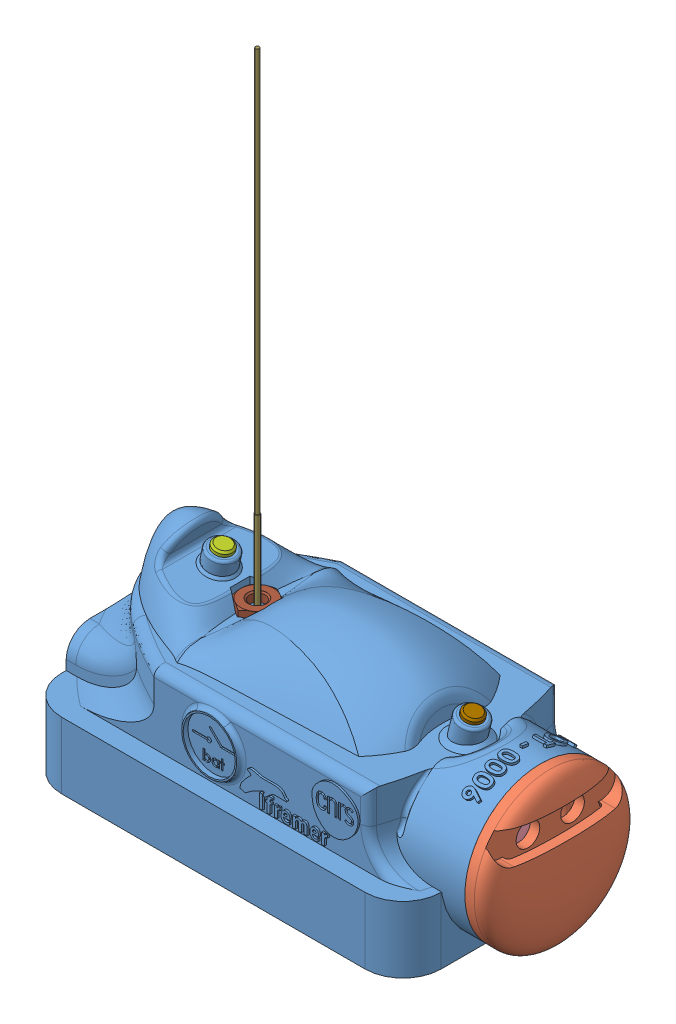
SolidWorks assembly Assemblage_iot_v.02.0, configuration Défaut. Lengths in mm.
Overall size (93.03 132.65 48).
16 component instances, 16 part files, 30 mates.
Components (placement in the parent):
- 0006-1: 0006 [Default] at (-51.4295 -21.1434 0) size (85.85 41.18 48)
- bouchon-1: bouchon [Défaut] at (-4.4295 -19.1434 -0.0066) x (-1 0 0) z (0 0 -1) size (15.85 32 32)
- IoT_Gnat-1: IoT_Gnat [Défaut] at (-25.1885 -16.3387 6.7757) x (-1 0 0) z (0 1 0) size (37.52 22.13 7.15)
- membrane-1: membrane [Défaut] at (-15.9295 -19.1434 -0.0066) x (0 0.019528 -0.999809) z (1 0 0) size (26.5 26.5 4)
- Passive_GPS_Antenna_uFL-15mm-15mm-1: Passive_GPS_Antenna_uFL-15mm-15mm [Défaut] at (-47.1795 -3.1434 -0.25) x (1 0 0) z (0 -1 0) size (15 15 7.3) (hidden)
- plan_de_masse-1: plan_de_masse [Défaut] at (-46.9295 -8.1434 0) x (0 0 -1) z (0 -1 0) size (30 40 2) (hidden)
- plaque_dessous-1: plaque_dessous [Défaut] at (-53.6795 -30.1434 -0.25) x (-1 0 0) z (0 -1 0) size (65.5 41.5 5)
- battery_1300mAh-1: battery_1300mAh [Défaut] at (-52.9295 -29.2621 0) size (60 5 37)
- socket button head screw_iso-1: socket button head screw_iso [ISO 7380 - M4 x 8 - 8N] at (-75.3695 -6.3142 0) x (0.207912 0.978148 0) z (0 0 1) size (10.2 7.6 7.6)
- 4pin_251-8351-1: 4pin_251-8351 [Défaut] at (-72.9295 -18.1529 -4.0779) x (0 1 0) z (1 0 0) size (2.5 10.16 20.94)
- socket countersunk head screw_iso-2: socket countersunk head screw_iso [ISO 10642 - M4 x 10 - 10N] at (-22.9456 -10.2399 0) x (0.241922 0.970296 0) z (0 0 1) size (10 7.53 7.53)
- bouchon_silicone-1: bouchon_silicone [Défaut] at (-91.4295 -18.1434 1) x (0 0 -1) z (1 0 0) size (15 6 10)
- hex thin nut chamfered gradeab_iso-1: hex thin nut chamfered gradeab_iso [ISO - 4035 - M4 - N] at (-66.3057 -5.1434 -0.1732) x (-0.5 0 -0.866025) z (0 -1 0) size (7 8.08 2.2)
- protec-1: protec [Défaut] at (-81.4841 -18.1262 0.0031) x (0 0 1) z (-1 0 0) size (14.7 5.8 40) (hidden)
- dock-1: dock [Défaut] at (-51.4295 -21.1434 0) x (1 0 0) z (0 1 0) size (29.08 48.15 28.26) (hidden)
- antenna_lora_V2-2: antenna_lora_V2 [Default] at (-66.3057 97.5027 -0.1732) x (-0.999787 0 0.020633) z (0.020633 0 0.999787) size (2 114.5 3)
Mates (geometry in assembly coordinates):
- Coaxiale1: concentric aligned: cylinder of 0006-1 through (-6.4295 -19.1434 -0.0066) axis (-1 0 0) radius 16; cylinder of membrane-1 through (-15.9295 -19.1434 -0.0066) axis (-1 0 0) radius 13.25
- Coïncidente1: coincident anti-aligned: plane of 0006-1 through (-15.9295 -19.1434 0) normal (1 0 0); plane of membrane-1 through (-15.9295 -5.8959 0.2522) normal (-1 0 0)
- Coaxiale2: concentric anti-aligned: cylinder of 0006-1 through (-6.4295 -19.1434 -0.0066) axis (-1 0 0) radius 16; cylinder of bouchon-1 through (-4.4295 -19.1434 -0.0066) axis (1 0 0) radius 16
- Parallèle1: parallel anti-aligned: plane of 0006-1 through (-6.742 -19.1434 13.9587) normal (0 -1 0); plane of bouchon-1 through (-6.742 -19.1434 13.4522) normal (0 1 0)
- Coïncidente3: coincident anti-aligned: plane of 0006-1 through (-6.4295 -19.1434 -0.0066) normal (1 0 0); plane of bouchon-1 through (-6.4295 -19.1434 -0.0066) normal (-1 0 0)
- Distance2: distance = 0.5 mm anti-aligned: plane of 0006-1 through (-55.1795 -2.1434 -8.25) normal (0 0 1); plane of Passive_GPS_Antenna_uFL-15mm-15mm-1 through (-54.6795 -8.1434 -7.75) normal (0 0 -1)
- Distance1: distance = 0.5 mm anti-aligned: plane of 0006-1 through (-55.1795 -2.1434 -8.25) normal (1 0 0); plane of Passive_GPS_Antenna_uFL-15mm-15mm-1 through (-54.6795 -8.1434 -7.75) normal (-1 0 0)
- Distance4: distance = 0.5 mm anti-aligned: plane of 0006-1 through (-84.9295 -23.1434 -19) normal (0 0 1); plane of battery_1300mAh-1 through (-82.9295 -24.2621 -18.5) normal (0 0 -1)
- Distance3: distance = 1 mm anti-aligned: plane of 0006-1 through (-21.9295 -23.1434 19) normal (-1 0 0); plane of battery_1300mAh-1 through (-22.9295 -24.2621 -18.5) normal (1 0 0)
- Coïncidente13: coincident aligned: plane of 0006-1 through (-51.4295 -35.1434 0) normal (0 -1 0); plane of plaque_dessous-1 through (-53.6795 -35.1434 -0.25) normal (0 -1 0)
- Coïncidente14: coincident anti-aligned: plane of 0006-1 through (-71.9295 -35.1434 -15) normal (0 0 1); plane of plan_de_masse-1 through (-66.9295 -10.1434 -15) normal (0 0 -1)
- Coïncidente15: coincident anti-aligned: plane of 0006-1 through (-26.9295 -35.1434 15) normal (-1 0 0); plane of plan_de_masse-1 through (-26.9295 -10.1434 15) normal (1 0 0)
- Coïncidente16: coincident anti-aligned: plane of 0006-1 through (-51.4295 -8.1434 0) normal (0 -1 0); plane of plan_de_masse-1 through (-46.9295 -8.1434 0) normal (0 1 0)
- Coïncidente20: coincident anti-aligned: plane of 0006-1 through (-86.4295 -30.1434 -21) normal (1 0 0); plane of plaque_dessous-1 through (-86.4295 -35.1434 -21) normal (-1 0 0)
- Coïncidente21: coincident anti-aligned: plane of 0006-1 through (-86.4295 -30.1434 -21) normal (0 0 1); plane of plaque_dessous-1 through (-20.9295 -35.1434 -21) normal (0 0 -1)
- Coaxiale3: concentric aligned: cylinder of 0006-1 through (-74.9121 -4.1623 0) axis (-0.207912 -0.978148 0) radius 4; cylinder of socket button head screw_iso-1 through (-75.3695 -6.3142 0) axis (-0.207912 -0.978148 0) radius 2
- Coïncidente22: coincident anti-aligned: plane of 0006-1 through (-74.9121 -4.1623 0) normal (-0.207912 -0.978148 0); plane of socket button head screw_iso-1 through (-76.8684 -3.7465 0) normal (0.207912 0.978148 0)
- Coïncidente24: coincident anti-aligned: plane of Passive_GPS_Antenna_uFL-15mm-15mm-1 through (-47.1795 -8.1434 -0.25) normal (0 -1 0); plane of plan_de_masse-1 through (-46.9295 -8.1434 0) normal (0 1 0)
- Coaxiale4: concentric anti-aligned: cylinder of 0006-1 through (-23.1924 -11.2296 0) axis (0.241922 0.970296 0) radius 3; cylinder of socket countersunk head screw_iso-2 through (-22.9456 -10.2399 0) axis (-0.241922 -0.970296 0) radius 2
- Coïncidente26: coincident aligned: cone of 0006-1 through (-22.8295 -9.7741 0) axis (0.241922 0.970296 0); cone of socket countersunk head screw_iso-2 through (-22.7727 -9.5461 0) axis (0.241922 0.970296 0)
- Coïncidente27: coincident anti-aligned: plane of 0006-1 through (-81.4295 -15.1434 -6.5) normal (0 -1 0); plane of bouchon_silicone-1 through (-81.4295 -15.1434 8.5) normal (0 1 0)
- Coïncidente28: coincident anti-aligned: plane of bouchon_silicone-1 through (-81.4295 -15.1434 -6.5) normal (0 0 -1); plane of 0006-1 through (-81.4295 -15.1434 -6.5) normal (0 0 1)
- Coïncidente29: coincident aligned: plane of 0006-1 through (-91.4295 -35.1434 -24) normal (-1 0 0); plane of bouchon_silicone-1 through (-91.4295 -18.1434 1) normal (-1 0 0)
- Coïncidente30: coincident anti-aligned: plane of 0006-1 through (-51.4295 -5.1434 0) normal (0 1 0); plane of hex thin nut chamfered gradeab_iso-1 through (-62.8057 -5.1434 5.889) normal (0 -1 0)
- Coïncidente31: coincident anti-aligned: plane of 0006-1 through (-69.8057 6.0333 -2.0785) normal (1 0 0); plane of hex thin nut chamfered gradeab_iso-1 through (-69.8057 -2.9434 1.8475) normal (-1 0 0)
- Coïncidente32: coincident anti-aligned: plane of 0006-1 through (-62.6057 6.0333 -2.0785) normal (-0.5 0 0.866025); plane of hex thin nut chamfered gradeab_iso-1 through (-66.3057 -2.9434 -4.2147) normal (0.5 0 -0.866025)
- Coïncidente34: coincident anti-aligned: plane of 0006-1 through (-51.4295 -21.1434 0) normal (0 1 0); plane of dock-1 through (-51.4295 -21.1434 0) normal (0 -1 0)
- Coïncidente35: coincident aligned: plane of 0006-1 through (-91.4295 -35.1434 -24) normal (0 0 -1); plane of dock-1 through (-56.4295 8.8566 -24) normal (0 0 -1)
- Coïncidente38: coincident: point of 0006-1; point of dock-1
- Coaxiale5: concentric anti-aligned: cylinder of hex thin nut chamfered gradeab_iso-1 through (-66.3057 -2.9434 -0.1732) axis (0 -1 0) radius 1.65; cylinder of antenna_lora_V2-2 through (-66.3057 -12.4973 -0.1732) axis (0 1 0) radius 0.5
